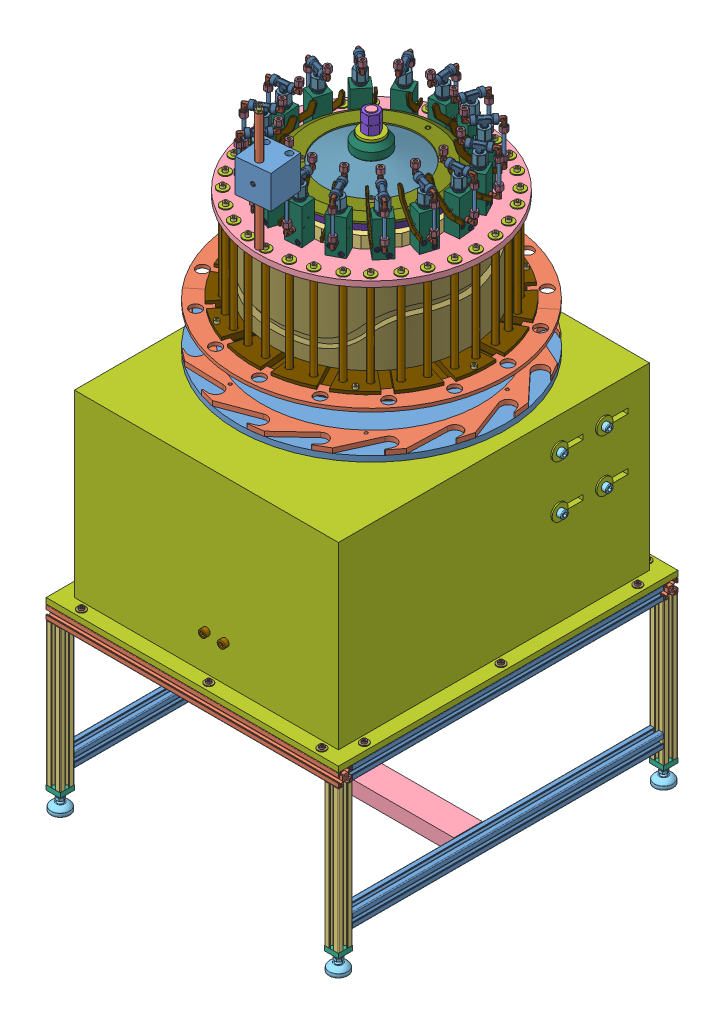
SolidWorks assembly Assieme_FINALE, configuration Default. Lengths in mm.
Overall size (1086.82 1425.57 1086.82).
701 component instances, 78 part files, 65 mates.
Components (placement in the parent):
- SupportoBase_Totale-2: SupportoBase_Totale [Default] at (4.0127 -14.4529 -3.9361) x (0 1 0) z (0 0 1) size (801.2 636.12 736.12)
  - Supporto_base_macchina-1: Supporto_base_macchina [Default] at origin size (378.2 636.12 736.12)
    - profilato_30x30_590-3: profilato_30x30_590 [Default] at (275.414 713.7262 -66.645) size (30 30 660)
    - profilato_30x30_590-5: profilato_30x30_590 [Default] at (275.414 123.7262 -66.645) size (30 30 660)
    - profilato_30x30_550-5: profilato_30x30_550 [Default] at (275.414 703.7262 -716.645) x (1 0 0) z (0 1 0) size (30 30 620)
    - profilato_30x30_550-6: profilato_30x30_550 [Default] at (275.414 703.7262 -26.645) x (1 0 0) z (0 1 0) size (30 30 620)
    - profilato_30x30_272-5: profilato_30x30_272 [Default] at (-16.586 123.7262 -716.645) x (0 0 1) z (-1 0 0) size (30 30 302)
    - profilato_30x30_272-6: profilato_30x30_272 [Default] at (-16.586 713.7262 -716.645) x (0 0 1) z (-1 0 0) size (30 30 302)
    - profilato_30x30_272-7: profilato_30x30_272 [Default] at (235.414 123.7262 -26.645) x (0 0 -1) z (1 0 0) size (30 30 302)
    - profilato_30x30_272-8: profilato_30x30_272 [Default] at (-16.586 713.7262 -26.645) x (0 0 1) z (-1 0 0) size (30 30 302)
    - profilo_U_60x30_490_supporto_base_macchina-1: profilo_U_60x30_490_supporto_base_macchina [Default] at (15.1 707.7262 -323.6583) x (0 0 1) z (0 -1 0) size (60 30 569)
    - profilato_30x30_590-6: profilato_30x30_590 [Default] at (3.414 123.7262 -66.645) size (30 30 660)
    - profilato_30x30_590-7: profilato_30x30_590 [Default] at (3.414 713.7262 -676.645) x (-1 0 0) z (0 0 -1) size (30 30 660)
    - 6322125-1: 6322125 [Default] at (-85.2818 713.7262 -26.645) x (0 0 -1) z (1 0 0) size (40 40 71.2)
    - 6322125-2: 6322125 [Default] at (-85.2818 713.7262 -716.645) x (0 0 -1) z (1 0 0) size (40 40 71.2)
    - 6322125-3: 6322125 [Default] at (-85.2818 123.7262 -26.645) x (0 -0.924225 -0.381849) z (1 0 0) size (40 40 71.2)
    - 6322125-4: 6322125 [Default] at (-85.2818 123.7262 -716.645) x (0 0 -1) z (1 0 0) size (40 40 71.2)
    - tappo_filettato_Supporto_base_macchina-1: tappo_filettato_Supporto_base_macchina [Default] at (-41.586 123.7262 -26.645) x (0 0 1) z (-1 0 0) size (30 30 10.37)
    - tappo_filettato_Supporto_base_macchina-2: tappo_filettato_Supporto_base_macchina [Default] at (-41.586 123.7262 -716.645) x (0 0 1) z (-1 0 0) size (30 30 10.37)
    - tappo_filettato_Supporto_base_macchina-3: tappo_filettato_Supporto_base_macchina [Default] at (-41.586 713.7262 -716.645) x (0 0 1) z (-1 0 0) size (30 30 10.37)
    - tappo_filettato_Supporto_base_macchina-4: tappo_filettato_Supporto_base_macchina [Default] at (-51.586 713.7262 -26.645) x (0 0 -1) z (1 0 0) size (30 30 10.37)
  - assieme_base-1: assieme_base [Default] at (466.8009 1138.7262 -472.0974) x (0 0 -1) z (0 -1 0) size (720 423 620)
    - Supporto di Base per macchina-1: Supporto di Base per macchina [Default] at (-460.4524 -176.3869 1030) size (720 403 620)
    - canotto di supporto-1: canotto di supporto [Default] at (-100.4524 134.8265 740) x (0 1 0) z (-0.866025 0 0.5) size (220 238 238)
    - m10 35mm-7: m10 35mm [ISO 4762 M10 x 35 - 35N] at (4.5476 246.6131 740) x (0 -1 0) z (1 0 0) size (45 16 16)
    - m10 35mm-8: m10 35mm [ISO 4762 M10 x 35 - 35N] at (-47.9524 246.6131 649.0673) x (0 -1 0) z (0.5 0 -0.866025) size (45 16 16)
    - m10 35mm-9: m10 35mm [ISO 4762 M10 x 35 - 35N] at (-152.9524 246.6131 649.0673) x (0 -1 0) z (-0.5 0 -0.866025) size (45 16 16)
    - m10 35mm-10: m10 35mm [ISO 4762 M10 x 35 - 35N] at (-205.4524 246.6131 740) x (0 -1 0) z (-1 0 0) size (45 16 16)
    - m10 35mm-11: m10 35mm [ISO 4762 M10 x 35 - 35N] at (-152.9524 246.6131 830.9327) x (0 -1 0) z (-0.5 0 0.866025) size (45 16 16)
    - m10 35mm-12: m10 35mm [ISO 4762 M10 x 35 - 35N] at (-47.9524 246.6131 830.9327) x (0 -1 0) z (0.5 0 0.866025) size (45 16 16)
    - Traversa di blocco albero-1: Traversa di blocco albero [Default] at (-100.4524 -86.3869 772.5) size (644 42 65)
    - m10 35mm-13: m10 35mm [ISO 4762 M10 x 35 - 35N] at (239.5476 -86.3869 760) x (-1 0 0) z (0 -1 0) size (45 16 16)
    - m10 35mm-16: m10 35mm [ISO 4762 M10 x 35 - 35N] at (239.5476 -86.3869 720) x (-1 0 0) z (0 -1 0) size (45 16 16)
    - m10 35mm-17: m10 35mm [ISO 4762 M10 x 35 - 35N] at (-440.4524 -86.3869 720) x (1 0 0) z (0 1 0) size (45 16 16)
    - m10 35mm-18: m10 35mm [ISO 4762 M10 x 35 - 35N] at (-440.4524 -86.3869 760) x (1 0 0) z (0 1 0) size (45 16 16)
  - DadoT-2: DadoT [Default] at (288.4104 668.7262 -716.645) x (0 0 -1) z (0 -1 0) size (16.5 6 8)
  - DadoT-9: DadoT [Default] at (288.4104 668.7262 -26.645) x (0 0 -1) z (0 -1 0) size (16.5 6 8)
  - DadoT-10: DadoT [Default] at (288.6104 713.7262 -661.645) x (0 1 0) z (0 0 -1) size (16.5 6 8)
  - DadoT-11: DadoT [Default] at (288.6104 713.7262 -371.645) x (0 1 0) z (0 0 -1) size (16.5 6 8)
  - DadoT-12: DadoT [Default] at (288.6104 713.7262 -81.645) x (0 1 0) z (0 0 -1) size (16.5 6 8)
  - DadoT-13: DadoT [Default] at (288.6104 123.7262 -661.645) x (0 1 0) z (0 0 -1) size (16.5 6 8)
  - DadoT-15: DadoT [Default] at (288.6104 123.7262 -371.645) x (0 1 0) z (0 0 -1) size (16.5 6 8)
  - DadoT-17: DadoT [Default] at (288.6104 123.7262 -81.645) x (0 1 0) z (0 0 -1) size (16.5 6 8)
  - RosettaM6-1: RosettaM6 [Washer ISO 7093 - 6] at (302.414 713.7262 -661.645) x (-1 0 0) z (0 0 1) size (1.6 18 18)
  - ViteM6-20-1: ViteM6-20 [ISO 4762 M6 x 20 - 20S] at (308.414 713.7262 -661.645) x (-1 0 0) z (0 0 1) size (26 10 10)
  - RosettaM6-2: RosettaM6 [Washer ISO 7093 - 6] at (302.414 668.7262 -716.645) x (-1 0 0) z (0 0 1) size (1.6 18 18)
  - ViteM6-20-2: ViteM6-20 [ISO 4762 M6 x 20 - 20S] at (308.414 668.7262 -716.645) x (-1 0 0) z (0 0 1) size (26 10 10)
  - RosettaM6-3: RosettaM6 [Washer ISO 7093 - 6] at (302.414 713.7262 -371.645) x (-1 0 0) z (0 0 1) size (1.6 18 18)
  - RosettaM6-4: RosettaM6 [Washer ISO 7093 - 6] at (302.414 713.7262 -81.645) x (-1 0 0) z (0 0 1) size (1.6 18 18)
  - ViteM6-20-3: ViteM6-20 [ISO 4762 M6 x 20 - 20S] at (308.414 713.7262 -371.645) x (-1 0 0) z (0 0 1) size (26 10 10)
  - ViteM6-20-4: ViteM6-20 [ISO 4762 M6 x 20 - 20S] at (308.414 713.7262 -81.645) x (-1 0 0) z (0 0 1) size (26 10 10)
  - RosettaM6-5: RosettaM6 [Washer ISO 7093 - 6] at (302.414 123.7262 -661.645) x (-1 0 0) z (0 0 1) size (1.6 18 18)
  - ViteM6-20-5: ViteM6-20 [ISO 4762 M6 x 20 - 20S] at (308.414 123.7262 -661.645) x (-1 0 0) z (0 0 1) size (26 10 10)
  - RosettaM6-6: RosettaM6 [Washer ISO 7093 - 6] at (302.414 123.7262 -371.645) x (-1 0 0) z (0 0 1) size (1.6 18 18)
  - RosettaM6-7: RosettaM6 [Washer ISO 7093 - 6] at (302.414 123.7262 -81.645) x (-1 0 0) z (0 0 1) size (1.6 18 18)
  - ViteM6-20-6: ViteM6-20 [ISO 4762 M6 x 20 - 20S] at (308.414 123.7262 -371.645) x (-1 0 0) z (0 0 1) size (26 10 10)
  - ViteM6-20-7: ViteM6-20 [ISO 4762 M6 x 20 - 20S] at (308.414 123.7262 -81.645) x (-1 0 0) z (0 0 1) size (26 10 10)
  - ViteM6-20-8: ViteM6-20 [ISO 4762 M6 x 20 - 20S] at (308.414 398.7262 -716.645) x (-1 0 0) z (0 0 1) size (26 10 10)
  - RosettaM6-8: RosettaM6 [Washer ISO 7093 - 6] at (302.414 398.7262 -716.645) x (-1 0 0) z (0 0 1) size (1.6 18 18)
  - DadoT-19: DadoT [Default] at (288.4104 398.7262 -716.645) x (0 0 -1) z (0 -1 0) size (16.5 6 8)
  - DadoT-20: DadoT [Default] at (288.4104 158.7262 -716.645) x (0 0 -1) z (0 -1 0) size (16.5 6 8)
  - RosettaM6-9: RosettaM6 [Washer ISO 7093 - 6] at (302.414 158.7262 -716.645) x (-1 0 0) z (0 0 1) size (1.6 18 18)
  - ViteM6-20-9: ViteM6-20 [ISO 4762 M6 x 20 - 20S] at (308.414 158.7262 -716.645) x (-1 0 0) z (0 0 1) size (26 10 10)
  - DadoT-21: DadoT [Default] at (288.4104 668.7262 -26.645) x (0 0 -1) z (0 -1 0) size (16.5 6 8)
  - RosettaM6-10: RosettaM6 [Washer ISO 7093 - 6] at (302.414 668.7262 -26.645) x (-1 0 0) z (0 0 1) size (1.6 18 18)
  - ViteM6-20-10: ViteM6-20 [ISO 4762 M6 x 20 - 20S] at (308.414 668.7262 -26.645) x (-1 0 0) z (0 0 1) size (26 10 10)
  - DadoT-22: DadoT [Default] at (288.4104 158.7262 -26.645) x (0 0 -1) z (0 -1 0) size (16.5 6 8)
  - RosettaM6-11: RosettaM6 [Washer ISO 7093 - 6] at (302.414 158.7262 -26.645) x (-1 0 0) z (0 0 1) size (1.6 18 18)
  - ViteM6-20-11: ViteM6-20 [ISO 4762 M6 x 20 - 20S] at (308.414 158.7262 -26.645) x (-1 0 0) z (0 0 1) size (26 10 10)
  - ViteM6-20-12: ViteM6-20 [ISO 4762 M6 x 20 - 20S] at (308.414 398.7262 -26.645) x (-1 0 0) z (0 0 1) size (26 10 10)
  - RosettaM6-12: RosettaM6 [Washer ISO 7093 - 6] at (302.414 398.7262 -26.645) x (-1 0 0) z (0 0 1) size (1.6 18 18)
  - DadoT-23: DadoT [Default] at (288.4104 398.7262 -26.645) x (0 0 -1) z (0 -1 0) size (16.5 6 8)
- motoriduttore-1: motoriduttore [Default] at (-164.7135 275.9611 -1137.0941) x (0 0 1) z (-1 0 0) size (200 160 175)
- Assieme_Riduttore-1: Assieme_Riduttore [Default] at (-58.5438 520.923 -522.9431) x (0 1 0) z (-0.993104 0 -0.117237) size (226 168.82 169.04)
  - AlberoRiduttore-1: AlberoRiduttore [Default] at (-61.6906 7.4655 211) size (201 29 29)
  - linguetta_uni6604_b_8x7x50-1: linguetta_uni6604_b_8x7x50 [Default] at (-116.7419 7.4655 226) x (1 0 0) z (0 1 0) size (50 7 8)
  - linguetta_uni6604_b_8x7x35-1: linguetta_uni6604_b_8x7x35 [Default] at (-33.7419 7.4655 226.5) x (1 0 0) z (0 1 0) size (35 7 8)
  - linguetta_uni6604_b_8x7x35-2: linguetta_uni6604_b_8x7x35 [Default] at (41.2581 7.4655 226.5) x (1 0 0) z (0 1 0) size (35 7 8)
  - ASSIEME-LASS-90-VERS-B-O-25-3D.step-1: ASSIEME-LASS-90-VERS-B-O-25-3D.step [Default] at (-111.3519 -70.5563 279.3493) x (-1 0 0) z (0 0.707107 -0.707107) size (64.28 105 105)
  - Rondella di fermo-1: Rondella di fermo [Default] at (-122.7419 7.4655 211) x (0 0.707107 -0.707107) z (-1 0 0) size (36 36 3)
  - M8 25 mm-1: M8 25 mm [ISO 4762 M8 x 25 - 25N] at (92.2581 7.4655 211) x (-1 0 0) z (0 1 0) size (33 13 13)
  - M8 25 mm-2: M8 25 mm [ISO 4762 M8 x 25 - 25N] at (-133.7419 7.4655 211) x (1 0 0) z (0 -0.707107 0.707107) size (33 13 13)
  - M6 16mm-3: M6 16mm [ISO 4762 M6 x 16 - 16N] at (-44.8119 40.5589 196.8286) x (-1 0 0) z (0 0.935687 0.352831) size (22 10 10)
  - M6 16mm-14: M6 16mm [ISO 4762 M6 x 16 - 16N] at (-44.8119 11.7394 175.2546) x (-1 0 0) z (0 0.773404 -0.633913) size (22 10 10)
  - M6 16mm-15: M6 16mm [ISO 4762 M6 x 16 - 16N] at (-44.8119 -21.354 189.426) x (-1 0 0) z (0 -0.162283 -0.986744) size (22 10 10)
  - M6 16mm-16: M6 16mm [ISO 4762 M6 x 16 - 16N] at (-44.8119 -25.6279 225.1714) x (-1 0 0) z (0 -0.935687 -0.352831) size (22 10 10)
  - M6 16mm-17: M6 16mm [ISO 4762 M6 x 16 - 16N] at (-44.8119 3.1916 246.7454) x (-1 0 0) z (0 -0.773404 0.633913) size (22 10 10)
  - M6 16mm-18: M6 16mm [ISO 4762 M6 x 16 - 16N] at (-44.8119 36.285 232.574) x (-1 0 0) z (0 0.162283 0.986744) size (22 10 10)
  - Parte1^Assieme_Riduttore-1: Parte1^Assieme_Riduttore [Default] at origin (virtual)
  - ruota dentata m22-4: ruota dentata m22 [Chain wheel ISO - 22Z 10A-1 --22SA36.0N] at (-59.7419 7.4655 211) x (1 0 0) z (0 -0.599278 0.800541) size (8.93 120.13 121.23)
  - Rondella di fermo-2: Rondella di fermo [Default] at (84.2581 7.4655 211) x (0 0 1) z (-1 0 0) size (36 36 3)
- M10 50mm-1: M10 50mm [ISO 4762 M10 x 50 - 50N] at (-121.7135 603.4611 -513.0941) x (-1 0 0) z (0 -0.924225 -0.381849) size (60 16 16)
- M10 50mm-2: M10 50mm [ISO 4762 M10 x 50 - 50N] at (-121.7135 492.4611 -513.0941) x (-1 0 0) z (0 0 1) size (60 16 16)
- M10 50mm-5: M10 50mm [ISO 4762 M10 x 50 - 50N] at (-121.7135 603.4611 -608.0941) x (-1 0 0) z (0 0 1) size (60 16 16)
- M10 50mm-4: M10 50mm [ISO 4762 M10 x 50 - 50N] at (-121.7135 492.4611 -608.0941) x (-1 0 0) z (0 0 1) size (60 16 16)
- DADO M10-9: DADO M10 [ISO - 4033 - M10 - W - N] at (-174.0135 603.4611 -608.0941) x (0 0 1) z (-1 0 0) size (16 18.48 9.3)
- DADO M10-8: DADO M10 [ISO - 4033 - M10 - W - N] at (-174.0135 603.4611 -513.0941) x (0 0 1) z (-1 0 0) size (16 18.48 9.3)
- DADO M10-7: DADO M10 [ISO - 4033 - M10 - W - N] at (-174.0135 492.4611 -608.0941) x (0 0 1) z (-1 0 0) size (16 18.48 9.3)
- DADO M10-10: DADO M10 [ISO - 4033 - M10 - W - N] at (-174.0135 492.4611 -513.0941) x (0 0 1) z (-1 0 0) size (16 18.48 9.3)
- rondella M10-9: rondella M10 [Washer ISO 7094 - 10] at (-134.7135 603.4611 -513.0941) x (-1 0 0) z (0 0.924225 0.381849) size (3 34 34)
- rondella M10-10: rondella M10 [Washer ISO 7094 - 10] at (-134.7135 492.4611 -513.0941) x (-1 0 0) z (0 0 1) size (3 34 34)
- rondella M10-12: rondella M10 [Washer ISO 7094 - 10] at (-134.7135 492.4611 -608.0941) x (-1 0 0) z (0 0 1) size (3 34 34)
- rondella M10-11: rondella M10 [Washer ISO 7094 - 10] at (-134.7135 603.4611 -608.0941) x (-1 0 0) z (0 0 1) size (3 34 34)
- catena_maschio-1: catena_maschio [Default] at (-321.9473 463.4961 -580.6395) x (-0.810007 0 0.58642) z (0 1 0) size (28.67 12.73 20.3)
- catena_femmina-1: catena_femmina [Default] at (-334.299 463.4961 -567.4631) x (0.810007 0 -0.58642) z (0 1 0) size (30.04 14.2 13.87)
  - ansi_50_02-1: ansi_50_02 [Default] at (17.7318 3.4296 0) x (1 0 0) z (0 0 -1) size (30.04 14.2 13.87)
  - ansi_50_03-1: ansi_50_03 [Default] at (17.7318 3.4296 -0.11) x (1 0 0) z (0 0 -1) size (10.16 10.16 9.46)
  - ansi_50_04-1: ansi_50_04 [Default] at (17.7318 3.4296 0.11) x (1 0 0) z (0 0 -1) size (10.16 10.16 9.46)
- rondella M8-1: rondella M8 [ISO 10673-9.3-S] at (-394.7135 376.9611 -360.5811) x (0 -1 0) z (-1 0 0) size (2 18 18)
- rondella M8-2: rondella M8 [ISO 10673-9.3-S] at (-394.7135 376.9611 -390.5811) x (0 -1 0) z (-1 0 0) size (2 18 18)
- M8 25 mm-1: M8 25 mm [ISO 4762 M8 x 25 - 25N] at (-394.7135 368.9611 -390.5811) x (0 1 0) z (0.5 0 0.866025) size (33 13 13)
- M8 25 mm-2: M8 25 mm [ISO 4762 M8 x 25 - 25N] at (-394.7135 366.9611 -360.5811) x (0 1 0) z (-0.5 0 -0.866025) size (33 13 13)
- assieme parte rotante-2: assieme parte rotante [Default] at (-79.201 623.9178 -645.7922) x (0 1 0) z (-0.73003 0 0.683415) size (749.63 778.63 778.63)
  - albero rotazione piatti-1: albero rotazione piatti [Default] at (60.413 18.3637 415) size (415 200 200)
  - seger 100mm-2: seger 100mm [KS 1336 E - 100] at (-146.4567 18.3637 415) x (0 0 -1) z (1 0 0) size (107.55 112.98 3)
  - SKF - 6020 - 20,DE,NC,20_68-1: SKF - 6020 - 20,DE,NC,20_68 [SKF - 6020 - 20,DE,NC,20_68] at (-131.4567 18.3637 415) x (1 0 0) z (0 -0.434476 -0.900684) size (24 150 150)
  - calettatore d95-1: calettatore d95 [Default] at (-173.8867 18.3637 415) size (39.5 135 135)
  - Chain wheel ISO - 50Z 10A-1-1: Chain wheel ISO - 50Z 10A-1 [Chain wheel ISO - 50Z 10A-1 --50SB120H25L95.0N] at (-164.8867 18.3637 415) size (28.93 262.06 262.51)
  - Disco supporto montaggio e Colonne-1: Disco supporto montaggio e Colonne [Default] at (204.0433 18.3637 415) x (0 -0.866025 -0.5) z (1 0 0) size (499.6 499.6 29)
  - SKF - 6020 - 20,DE,NC,20_68-2: SKF - 6020 - 20,DE,NC,20_68 [SKF - 6020 - 20,DE,NC,20_68] at (62.0433 18.3637 415) x (1 0 0) z (0 -0.432628 -0.901573) size (24 150 150)
  - piatto rotante porta tappi-1: piatto rotante porta tappi [Default] at (99.0433 18.3637 415) x (0 0 -1) z (1 0 0) size (570 570 20.57)
  - disco trasportatore tappi 31-1: disco trasportatore tappi 31 [Default] at (111.0433 18.3637 415) x (0 0.5 -0.866025) z (1 0 0) size (570 570 10.42)
  - Distributore Rotante-1: Distributore Rotante [Default] at (425.0433 18.3637 415) x (0 0.130526 -0.991445) z (1 0 0) size (310 310 25.54)
  - disco trascinato porta distributore vuoto-1: disco trascinato porta distributore vuoto [Default] at (400.0433 18.3637 415) x (0 -0.130526 0.991445) z (-1 0 0) size (480 480 50)
  - m12 35mm-1: m12 35mm [ISO 4762 M12 x 35 - 35N] at (376.0433 -45.1046 366.2991) x (1 0 0) z (0 -0.5 0.866025) size (47 18 18)
  - m12 90mm-3: m12 90mm [ISO 4762 M12 x 90 - 90N] at (203.0433 -21.6363 345.718) x (-1 0 0) z (0 -0.5 0.866025) size (102 18 18)
  - rondella M6-90: rondella M6 [Washer ISO 7094 - 6] at (99.0433 -101.6363 207.1539) x (1 0 0) z (0 -1 0) size (2 22 22)
  - M6 20mm-1: M6 20mm [ISO 4762 M6 x 20 - 20N] at (91.0433 -101.6363 207.1539) x (1 0 0) z (0 0.5 0.866025) size (26 10 10)
  - m12 35mm-2: m12 35mm [ISO 4762 M12 x 35 - 35N] at (376.0433 28.8058 335.6844) x (1 0 0) z (0 -1 0) size (47 18 18)
  - m12 35mm-3: m12 35mm [ISO 4762 M12 x 35 - 35N] at (376.0433 92.2741 384.3853) x (1 0 0) z (0 -0.5 -0.866025) size (47 18 18)
  - m12 35mm-4: m12 35mm [ISO 4762 M12 x 35 - 35N] at (376.0433 81.832 463.7009) x (1 0 0) z (0 0.5 -0.866025) size (47 18 18)
  - m12 35mm-5: m12 35mm [ISO 4762 M12 x 35 - 35N] at (376.0433 7.9216 494.3156) x (1 0 0) z (0 1 0) size (47 18 18)
  - m12 35mm-6: m12 35mm [ISO 4762 M12 x 35 - 35N] at (376.0433 -55.5467 445.6147) x (1 0 0) z (0 0.5 0.866025) size (47 18 18)
  - rondella M6-91: rondella M6 [Washer ISO 7094 - 6] at (99.0433 138.3637 207.1539) x (1 0 0) z (0 -0.5 -0.866025) size (2 22 22)
  - rondella M6-92: rondella M6 [Washer ISO 7094 - 6] at (99.0433 258.3637 415) x (1 0 0) z (0 0.5 -0.866025) size (2 22 22)
  - rondella M6-93: rondella M6 [Washer ISO 7094 - 6] at (99.0433 138.3637 622.8461) x (1 0 0) z (0 1 0) size (2 22 22)
  - rondella M6-94: rondella M6 [Washer ISO 7094 - 6] at (99.0433 -101.6363 622.8461) x (1 0 0) z (0 0.5 0.866025) size (2 22 22)
  - rondella M6-95: rondella M6 [Washer ISO 7094 - 6] at (99.0433 -221.6363 415) x (1 0 0) z (0 -0.5 0.866025) size (2 22 22)
  - M6 20mm-2: M6 20mm [ISO 4762 M6 x 20 - 20N] at (91.0433 138.3637 207.1539) x (1 0 0) z (0 -0.5 0.866025) size (26 10 10)
  - M6 20mm-3: M6 20mm [ISO 4762 M6 x 20 - 20N] at (91.0433 258.3637 415) x (1 0 0) z (0 -1 0) size (26 10 10)
  - M6 20mm-4: M6 20mm [ISO 4762 M6 x 20 - 20N] at (91.0433 138.3637 622.8461) x (1 0 0) z (0 -0.5 -0.866025) size (26 10 10)
  - M6 20mm-5: M6 20mm [ISO 4762 M6 x 20 - 20N] at (91.0433 -101.6363 622.8461) x (1 0 0) z (0 0.5 -0.866025) size (26 10 10)
  - M6 20mm-6: M6 20mm [ISO 4762 M6 x 20 - 20N] at (91.0433 -221.6363 415) x (1 0 0) z (0 1 0) size (26 10 10)
  - m12 90mm-4: m12 90mm [ISO 4762 M12 x 90 - 90N] at (203.0433 58.3637 345.718) x (-1 0 0) z (0 -1 0) size (102 18 18)
  - m12 90mm-5: m12 90mm [ISO 4762 M12 x 90 - 90N] at (203.0433 98.3637 415) x (-1 0 0) z (0 -0.5 -0.866025) size (102 18 18)
  - m12 90mm-6: m12 90mm [ISO 4762 M12 x 90 - 90N] at (203.0433 58.3637 484.282) x (-1 0 0) z (0 0.5 -0.866025) size (102 18 18)
  - m12 90mm-7: m12 90mm [ISO 4762 M12 x 90 - 90N] at (203.0433 -21.6363 484.282) x (-1 0 0) z (0 1 0) size (102 18 18)
  - m12 90mm-8: m12 90mm [ISO 4762 M12 x 90 - 90N] at (203.0433 -61.6363 415) x (-1 0 0) z (0 0.5 0.866025) size (102 18 18)
  - asta scorrimento carello-1: asta scorrimento carello [Default] at (287.5433 70.1437 197.9013) x (0 0 -1) z (1 0 0) size (12 12 225)
  - rondella M6-74: rondella M6 [Washer ISO 7094 - 6] at (175.0433 70.1437 197.9013) x (1 0 0) z (0 -1 0) size (2 22 22)
  - M6 16mm-1: M6 16mm [ISO 4762 M6 x 16 - 16N] at (167.0433 70.1437 197.9013) size (22 10 10)
  - M6 16mm-2: M6 16mm [ISO 4762 M6 x 16 - 16N] at (408.0433 70.1437 197.9013) x (-1 0 0) z (0 0 -1) size (22 10 10)
  - rondella M6-96: rondella M6 [Washer ISO 7094 - 6] at (400.0433 70.1437 197.9013) x (-1 0 0) z (0 1 0) size (2 22 22)
  - rondella M6-112: rondella M6 [Washer ISO 7094 - 6] at (175.0433 24.5373 191.8971) x (1 0 0) z (0 -0.965926 -0.258819) size (2 22 22)
  - M6 16mm-3: M6 16mm [ISO 4762 M6 x 16 - 16N] at (167.0433 24.5373 191.8971) x (1 0 0) z (0 0.258819 -0.965926) size (22 10 10)
  - asta scorrimento carello-2: asta scorrimento carello [Default] at (287.5433 24.5373 191.8971) x (0 0.258819 -0.965926) z (-1 0 0) size (12 12 225)
  - rondella M6-128: rondella M6 [Washer ISO 7094 - 6] at (400.0433 24.5373 191.8971) x (-1 0 0) z (0 0.965926 0.258819) size (2 22 22)
  - M6 16mm-4: M6 16mm [ISO 4762 M6 x 16 - 16N] at (408.0433 24.5373 191.8971) x (-1 0 0) z (0 -0.258819 0.965926) size (22 10 10)
  - AssiemeValvola-1: AssiemeValvola [Default] at (515.3257 103.3637 267.7757) x (0 -0.5 0.866025) z (0 0.866025 0.5) size (90.26 138.63 38)
    - RaccordoT-1: RaccordoT [Default] at origin size (43 29.75 16.5)
    - Raccordo a L-1: Raccordo a L [Default] at (-30 0 0) x (0 -1 0) z (0 0 -1) size (28.34 25.51 14.01)
      - 1809_06_10_01-1: 1809_06_10_01 [Default] at origin size (22.49 23 10)
      - 1809_06_10_02-1: 1809_06_10_02 [Default] at origin size (6.5 8.5 8.5)
      - 1809_06_10_03-1: 1809_06_10_03 [Default] at origin size (11.02 15.01 14.01)
    - Raccordo a L-2: Raccordo a L [Default] at (30 0 0) x (0 1 0) z (0 0 -1) size (28.34 25.51 14.01)
      - 1809_06_10_01-1: 1809_06_10_01 [Default] at origin size (22.49 23 10)
      - 1809_06_10_02-1: 1809_06_10_02 [Default] at origin size (6.5 8.5 8.5)
      - 1809_06_10_03-1: 1809_06_10_03 [Default] at origin size (11.02 15.01 14.01)
    - TappoChiusura-1: TappoChiusura [Default] at (0 -32 0) x (0 -1 0) z (0 0 1) size (38.28 26.74 26.74)
    - CorpoValvola-1: CorpoValvola [Default] at (-15 -115.2824 0) size (30 75 34)
    - Raccordo a L-3: Raccordo a L [Default] at (-30 -88.2824 0) x (0 1 0) z (0 0 1) size (28.34 25.51 14.01)
      - 1809_06_10_01-1: 1809_06_10_01 [Default] at origin size (22.49 23 10)
      - 1809_06_10_02-1: 1809_06_10_02 [Default] at origin size (6.5 8.5 8.5)
      - 1809_06_10_03-1: 1809_06_10_03 [Default] at origin size (11.02 15.01 14.01)
    - Spina_3x38-1: Spina_3x38 [Default] at (0 -68.2824 -21) x (-1 0 0) z (0 0 1) size (3 3 38)
    - Spina_3x38-2: Spina_3x38 [Default] at (-10 -80.2824 -21) x (0.996193 0.087174 0) z (0 0 1) size (3 3 38)
    - M5 40mm-3: M5 40mm [ISO 4762 M5 x 40 - 40N] at (-14.6 -108.7824 9) size (45 8.5 8.5)
    - M5 40mm-2: M5 40mm [ISO 4762 M5 x 40 - 40N] at (-14.6 -96.7824 -9) size (45 8.5 8.5)
    - LevaValvola-1: LevaValvola [Default] at (-24.507 -86.571 -17) x (0.996193 0.087174 0) z (0 0 1) size (77.55 60.2 4)
    - Tubo-1: Tubo [Default] at (-30 -15.9665 0) x (1 0 0) z (0 -1 0) size (6 6 56.4)
  - M6 16mm-5: M6 16mm [ISO 4762 M6 x 16 - 16N] at (167.0433 -16.8778 194.6116) x (1 0 0) z (0 0.382683 0.92388) size (22 10 10)
  - M6 16mm-6: M6 16mm [ISO 4762 M6 x 16 - 16N] at (167.0433 -98.5342 224.874) x (1 0 0) z (0 0.707107 0.707107) size (22 10 10)
  - M6 16mm-7: M6 16mm [ISO 4762 M6 x 16 - 16N] at (167.0433 -162.3939 284.0814) x (1 0 0) z (0 0.92388 0.382683) size (22 10 10)
  - M6 16mm-8: M6 16mm [ISO 4762 M6 x 16 - 16N] at (167.0433 -198.735 363.22) x (1 0 0) z (0 1 0) size (22 10 10)
  - M6 16mm-9: M6 16mm [ISO 4762 M6 x 16 - 16N] at (167.0433 -202.0247 450.2415) x (1 0 0) z (0 0.92388 -0.382683) size (22 10 10)
  - M6 16mm-10: M6 16mm [ISO 4762 M6 x 16 - 16N] at (167.0433 -171.7623 531.8979) x (1 0 0) z (0 0.707107 -0.707107) size (22 10 10)
  - M6 16mm-11: M6 16mm [ISO 4762 M6 x 16 - 16N] at (167.0433 -112.5549 595.7576) x (1 0 0) z (0 0.382683 -0.92388) size (22 10 10)
  - M6 16mm-12: M6 16mm [ISO 4762 M6 x 16 - 16N] at (167.0433 -33.4163 632.0987) x (1 0 0) z (0 0 -1) size (22 10 10)
  - M6 16mm-13: M6 16mm [ISO 4762 M6 x 16 - 16N] at (167.0433 53.6052 635.3884) x (1 0 0) z (0 -0.382683 -0.92388) size (22 10 10)
  - M6 16mm-14: M6 16mm [ISO 4762 M6 x 16 - 16N] at (167.0433 135.2616 605.126) x (1 0 0) z (0 -0.707107 -0.707107) size (22 10 10)
  - M6 16mm-15: M6 16mm [ISO 4762 M6 x 16 - 16N] at (167.0433 199.1213 545.9186) x (1 0 0) z (0 -0.92388 -0.382683) size (22 10 10)
  - M6 16mm-16: M6 16mm [ISO 4762 M6 x 16 - 16N] at (167.0433 235.4624 466.78) x (1 0 0) z (0 -1 0) size (22 10 10)
  - M6 16mm-17: M6 16mm [ISO 4762 M6 x 16 - 16N] at (167.0433 238.7521 379.7585) x (1 0 0) z (0 -0.92388 0.382683) size (22 10 10)
  - M6 16mm-18: M6 16mm [ISO 4762 M6 x 16 - 16N] at (167.0433 208.4897 298.1021) x (1 0 0) z (0 -0.707107 0.707107) size (22 10 10)
  - M6 16mm-19: M6 16mm [ISO 4762 M6 x 16 - 16N] at (167.0433 149.2823 234.2424) x (1 0 0) z (0 -0.382683 0.92388) size (22 10 10)
  - rondella M6-75: rondella M6 [Washer ISO 7094 - 6] at (175.0433 -16.8778 194.6116) x (1 0 0) z (0 -0.92388 0.382683) size (2 22 22)
  - rondella M6-76: rondella M6 [Washer ISO 7094 - 6] at (175.0433 -98.5342 224.874) x (1 0 0) z (0 -0.707107 0.707107) size (2 22 22)
  - rondella M6-77: rondella M6 [Washer ISO 7094 - 6] at (175.0433 -162.3939 284.0814) x (1 0 0) z (0 -0.382683 0.92388) size (2 22 22)
  - rondella M6-78: rondella M6 [Washer ISO 7094 - 6] at (175.0433 -198.735 363.22) size (2 22 22)
  - rondella M6-79: rondella M6 [Washer ISO 7094 - 6] at (175.0433 -202.0247 450.2415) x (1 0 0) z (0 0.382683 0.92388) size (2 22 22)
  - rondella M6-80: rondella M6 [Washer ISO 7094 - 6] at (175.0433 -171.7623 531.8979) x (1 0 0) z (0 0.707107 0.707107) size (2 22 22)
  - rondella M6-81: rondella M6 [Washer ISO 7094 - 6] at (175.0433 -112.5549 595.7576) x (1 0 0) z (0 0.92388 0.382683) size (2 22 22)
  - rondella M6-82: rondella M6 [Washer ISO 7094 - 6] at (175.0433 -33.4163 632.0987) x (1 0 0) z (0 1 0) size (2 22 22)
  - rondella M6-83: rondella M6 [Washer ISO 7094 - 6] at (175.0433 53.6052 635.3884) x (1 0 0) z (0 0.92388 -0.382683) size (2 22 22)
  - rondella M6-84: rondella M6 [Washer ISO 7094 - 6] at (175.0433 135.2616 605.126) x (1 0 0) z (0 0.707107 -0.707107) size (2 22 22)
  - rondella M6-85: rondella M6 [Washer ISO 7094 - 6] at (175.0433 199.1213 545.9186) x (1 0 0) z (0 0.382683 -0.92388) size (2 22 22)
  - rondella M6-86: rondella M6 [Washer ISO 7094 - 6] at (175.0433 235.4624 466.78) x (1 0 0) z (0 0 -1) size (2 22 22)
  - rondella M6-87: rondella M6 [Washer ISO 7094 - 6] at (175.0433 238.7521 379.7585) x (1 0 0) z (0 -0.382683 -0.92388) size (2 22 22)
  - rondella M6-88: rondella M6 [Washer ISO 7094 - 6] at (175.0433 208.4897 298.1021) x (1 0 0) z (0 -0.707107 -0.707107) size (2 22 22)
  - rondella M6-89: rondella M6 [Washer ISO 7094 - 6] at (175.0433 149.2823 234.2424) x (1 0 0) z (0 -0.92388 -0.382683) size (2 22 22)
  - asta scorrimento carello-3: asta scorrimento carello [Default] at (287.5433 -16.8778 194.6116) x (0 -0.382683 -0.92388) z (1 0 0) size (12 12 225)
  - asta scorrimento carello-4: asta scorrimento carello [Default] at (287.5433 -98.5342 224.874) x (0 -0.707107 -0.707107) z (1 0 0) size (12 12 225)
  - asta scorrimento carello-5: asta scorrimento carello [Default] at (287.5433 -162.3939 284.0814) x (0 -0.92388 -0.382683) z (1 0 0) size (12 12 225)
  - asta scorrimento carello-6: asta scorrimento carello [Default] at (287.5433 -198.735 363.22) x (0 -1 0) z (1 0 0) size (12 12 225)
  - asta scorrimento carello-7: asta scorrimento carello [Default] at (287.5433 -202.0247 450.2415) x (0 -0.92388 0.382683) z (1 0 0) size (12 12 225)
  - asta scorrimento carello-8: asta scorrimento carello [Default] at (287.5433 -171.7623 531.8979) x (0 -0.707107 0.707107) z (1 0 0) size (12 12 225)
  - asta scorrimento carello-9: asta scorrimento carello [Default] at (287.5433 -112.5549 595.7576) x (0 -0.382683 0.92388) z (1 0 0) size (12 12 225)
  - asta scorrimento carello-10: asta scorrimento carello [Default] at (287.5433 -33.4163 632.0987) x (0 0 1) z (1 0 0) size (12 12 225)
  - asta scorrimento carello-11: asta scorrimento carello [Default] at (287.5433 53.6052 635.3884) x (0 0.382683 0.92388) z (1 0 0) size (12 12 225)
  - asta scorrimento carello-12: asta scorrimento carello [Default] at (287.5433 135.2616 605.126) x (0 0.707107 0.707107) z (1 0 0) size (12 12 225)
  - asta scorrimento carello-13: asta scorrimento carello [Default] at (287.5433 199.1213 545.9186) x (0 0.92388 0.382683) z (1 0 0) size (12 12 225)
  - asta scorrimento carello-14: asta scorrimento carello [Default] at (287.5433 235.4624 466.78) x (0 1 0) z (1 0 0) size (12 12 225)
  - asta scorrimento carello-15: asta scorrimento carello [Default] at (287.5433 238.7521 379.7585) x (0 0.92388 -0.382683) z (1 0 0) size (12 12 225)
  - asta scorrimento carello-16: asta scorrimento carello [Default] at (287.5433 208.4897 298.1021) x (0 0.707107 -0.707107) z (1 0 0) size (12 12 225)
  - asta scorrimento carello-17: asta scorrimento carello [Default] at (287.5433 149.2823 234.2424) x (0 0.382683 -0.92388) z (1 0 0) size (12 12 225)
  - M6 16mm-20: M6 16mm [ISO 4762 M6 x 16 - 16N] at (408.0433 -16.8778 194.6116) x (-1 0 0) z (0 -0.382683 -0.92388) size (22 10 10)
  - M6 16mm-21: M6 16mm [ISO 4762 M6 x 16 - 16N] at (408.0433 -98.5342 224.874) x (-1 0 0) z (0 -0.707107 -0.707107) size (22 10 10)
  - M6 16mm-22: M6 16mm [ISO 4762 M6 x 16 - 16N] at (408.0433 -162.3939 284.0814) x (-1 0 0) z (0 -0.92388 -0.382683) size (22 10 10)
  - M6 16mm-23: M6 16mm [ISO 4762 M6 x 16 - 16N] at (408.0433 -198.735 363.22) x (-1 0 0) z (0 -1 0) size (22 10 10)
  - M6 16mm-24: M6 16mm [ISO 4762 M6 x 16 - 16N] at (408.0433 -202.0247 450.2415) x (-1 0 0) z (0 -0.92388 0.382683) size (22 10 10)
  - M6 16mm-25: M6 16mm [ISO 4762 M6 x 16 - 16N] at (408.0433 -171.7623 531.8979) x (-1 0 0) z (0 -0.707107 0.707107) size (22 10 10)
  - M6 16mm-26: M6 16mm [ISO 4762 M6 x 16 - 16N] at (408.0433 -112.5549 595.7576) x (-1 0 0) z (0 -0.382683 0.92388) size (22 10 10)
  - M6 16mm-27: M6 16mm [ISO 4762 M6 x 16 - 16N] at (408.0433 -33.4163 632.0987) x (-1 0 0) z (0 0 1) size (22 10 10)
  - M6 16mm-28: M6 16mm [ISO 4762 M6 x 16 - 16N] at (408.0433 53.6052 635.3884) x (-1 0 0) z (0 0.382683 0.92388) size (22 10 10)
  - M6 16mm-29: M6 16mm [ISO 4762 M6 x 16 - 16N] at (408.0433 135.2616 605.126) x (-1 0 0) z (0 0.707107 0.707107) size (22 10 10)
  - M6 16mm-30: M6 16mm [ISO 4762 M6 x 16 - 16N] at (408.0433 199.1213 545.9186) x (-1 0 0) z (0 0.92388 0.382683) size (22 10 10)
  - M6 16mm-31: M6 16mm [ISO 4762 M6 x 16 - 16N] at (408.0433 235.4624 466.78) x (-1 0 0) z (0 1 0) size (22 10 10)
  - M6 16mm-32: M6 16mm [ISO 4762 M6 x 16 - 16N] at (408.0433 238.7521 379.7585) x (-1 0 0) z (0 0.92388 -0.382683) size (22 10 10)
  - M6 16mm-33: M6 16mm [ISO 4762 M6 x 16 - 16N] at (408.0433 208.4897 298.1021) x (-1 0 0) z (0 0.707107 -0.707107) size (22 10 10)
  - M6 16mm-34: M6 16mm [ISO 4762 M6 x 16 - 16N] at (408.0433 149.2823 234.2424) x (-1 0 0) z (0 0.382683 -0.92388) size (22 10 10)
  - rondella M6-97: rondella M6 [Washer ISO 7094 - 6] at (400.0433 -16.8778 194.6116) x (-1 0 0) z (0 0.92388 -0.382683) size (2 22 22)
  - rondella M6-98: rondella M6 [Washer ISO 7094 - 6] at (400.0433 -98.5342 224.874) x (-1 0 0) z (0 0.707107 -0.707107) size (2 22 22)
  - rondella M6-99: rondella M6 [Washer ISO 7094 - 6] at (400.0433 -162.3939 284.0814) x (-1 0 0) z (0 0.382683 -0.92388) size (2 22 22)
  - rondella M6-100: rondella M6 [Washer ISO 7094 - 6] at (400.0433 -198.735 363.22) x (-1 0 0) z (0 0 -1) size (2 22 22)
  - rondella M6-101: rondella M6 [Washer ISO 7094 - 6] at (400.0433 -202.0247 450.2415) x (-1 0 0) z (0 -0.382683 -0.92388) size (2 22 22)
  - rondella M6-102: rondella M6 [Washer ISO 7094 - 6] at (400.0433 -171.7623 531.8979) x (-1 0 0) z (0 -0.707107 -0.707107) size (2 22 22)
  - rondella M6-103: rondella M6 [Washer ISO 7094 - 6] at (400.0433 -112.5549 595.7576) x (-1 0 0) z (0 -0.92388 -0.382683) size (2 22 22)
  - rondella M6-104: rondella M6 [Washer ISO 7094 - 6] at (400.0433 -33.4163 632.0987) x (-1 0 0) z (0 -1 0) size (2 22 22)
  - rondella M6-105: rondella M6 [Washer ISO 7094 - 6] at (400.0433 53.6052 635.3884) x (-1 0 0) z (0 -0.92388 0.382683) size (2 22 22)
  - rondella M6-106: rondella M6 [Washer ISO 7094 - 6] at (400.0433 135.2616 605.126) x (-1 0 0) z (0 -0.707107 0.707107) size (2 22 22)
  - rondella M6-107: rondella M6 [Washer ISO 7094 - 6] at (400.0433 199.1213 545.9186) x (-1 0 0) z (0 -0.382683 0.92388) size (2 22 22)
  - rondella M6-108: rondella M6 [Washer ISO 7094 - 6] at (400.0433 235.4624 466.78) x (-1 0 0) z (0 0 1) size (2 22 22)
  - rondella M6-109: rondella M6 [Washer ISO 7094 - 6] at (400.0433 238.7521 379.7585) x (-1 0 0) z (0 0.382683 0.92388) size (2 22 22)
  - rondella M6-110: rondella M6 [Washer ISO 7094 - 6] at (400.0433 208.4897 298.1021) x (-1 0 0) z (0 0.707107 0.707107) size (2 22 22)
  - rondella M6-111: rondella M6 [Washer ISO 7094 - 6] at (400.0433 149.2823 234.2424) x (-1 0 0) z (0 0.92388 0.382683) size (2 22 22)
  - rondella M6-113: rondella M6 [Washer ISO 7094 - 6] at (175.0433 -61.3104 206.5173) x (1 0 0) z (0 -0.991445 0.130526) size (2 22 22)
  - rondella M6-114: rondella M6 [Washer ISO 7094 - 6] at (175.0433 -135.0285 252.8771) x (1 0 0) z (0 -0.866025 0.5) size (2 22 22)
  - rondella M6-115: rondella M6 [Washer ISO 7094 - 6] at (175.0433 -185.3939 323.9186) x (1 0 0) z (0 -0.608761 0.793353) size (2 22 22)
  - rondella M6-116: rondella M6 [Washer ISO 7094 - 6] at (175.0433 -204.7392 408.8264) x (1 0 0) z (0 -0.258819 0.965926) size (2 22 22)
  - rondella M6-117: rondella M6 [Washer ISO 7094 - 6] at (175.0433 -190.119 494.6741) x (1 0 0) z (0 0.130526 0.991445) size (2 22 22)
  - rondella M6-118: rondella M6 [Washer ISO 7094 - 6] at (175.0433 -143.7592 568.3922) x (1 0 0) z (0 0.5 0.866025) size (2 22 22)
  - rondella M6-119: rondella M6 [Washer ISO 7094 - 6] at (175.0433 -72.7177 618.7576) x (1 0 0) z (0 0.793353 0.608761) size (2 22 22)
  - rondella M6-120: rondella M6 [Washer ISO 7094 - 6] at (175.0433 12.1901 638.1029) x (1 0 0) z (0 0.965926 0.258819) size (2 22 22)
  - rondella M6-121: rondella M6 [Washer ISO 7094 - 6] at (175.0433 98.0378 623.4827) x (1 0 0) z (0 0.991445 -0.130526) size (2 22 22)
  - rondella M6-122: rondella M6 [Washer ISO 7094 - 6] at (175.0433 171.7559 577.1229) x (1 0 0) z (0 0.866025 -0.5) size (2 22 22)
  - rondella M6-123: rondella M6 [Washer ISO 7094 - 6] at (175.0433 222.1213 506.0814) x (1 0 0) z (0 0.608761 -0.793353) size (2 22 22)
  - rondella M6-124: rondella M6 [Washer ISO 7094 - 6] at (175.0433 241.4666 421.1736) x (1 0 0) z (0 0.258819 -0.965926) size (2 22 22)
  - rondella M6-125: rondella M6 [Washer ISO 7094 - 6] at (175.0433 226.8464 335.3259) x (1 0 0) z (0 -0.130526 -0.991445) size (2 22 22)
  - rondella M6-126: rondella M6 [Washer ISO 7094 - 6] at (175.0433 180.4866 261.6078) x (1 0 0) z (0 -0.5 -0.866025) size (2 22 22)
  - rondella M6-127: rondella M6 [Washer ISO 7094 - 6] at (175.0433 109.4451 211.2424) x (1 0 0) z (0 -0.793353 -0.608761) size (2 22 22)
  - M6 16mm-35: M6 16mm [ISO 4762 M6 x 16 - 16N] at (167.0433 -61.3104 206.5173) x (1 0 0) z (0 -0.130526 -0.991445) size (22 10 10)
  - M6 16mm-36: M6 16mm [ISO 4762 M6 x 16 - 16N] at (167.0433 -135.0285 252.8771) x (1 0 0) z (0 -0.5 -0.866025) size (22 10 10)
  - M6 16mm-37: M6 16mm [ISO 4762 M6 x 16 - 16N] at (167.0433 -185.3939 323.9186) x (1 0 0) z (0 -0.793353 -0.608761) size (22 10 10)
  - M6 16mm-38: M6 16mm [ISO 4762 M6 x 16 - 16N] at (167.0433 -204.7392 408.8264) x (1 0 0) z (0 -0.965926 -0.258819) size (22 10 10)
  - M6 16mm-39: M6 16mm [ISO 4762 M6 x 16 - 16N] at (167.0433 -190.119 494.6741) x (1 0 0) z (0 -0.991445 0.130526) size (22 10 10)
  - M6 16mm-40: M6 16mm [ISO 4762 M6 x 16 - 16N] at (167.0433 -143.7592 568.3922) x (1 0 0) z (0 -0.866025 0.5) size (22 10 10)
  - M6 16mm-41: M6 16mm [ISO 4762 M6 x 16 - 16N] at (167.0433 -72.7177 618.7576) x (1 0 0) z (0 -0.608761 0.793353) size (22 10 10)
  - M6 16mm-42: M6 16mm [ISO 4762 M6 x 16 - 16N] at (167.0433 12.1901 638.1029) x (1 0 0) z (0 -0.258819 0.965926) size (22 10 10)
  - M6 16mm-43: M6 16mm [ISO 4762 M6 x 16 - 16N] at (167.0433 98.0378 623.4827) x (1 0 0) z (0 0.130526 0.991445) size (22 10 10)
  - M6 16mm-44: M6 16mm [ISO 4762 M6 x 16 - 16N] at (167.0433 171.7559 577.1229) x (1 0 0) z (0 0.5 0.866025) size (22 10 10)
  - M6 16mm-45: M6 16mm [ISO 4762 M6 x 16 - 16N] at (167.0433 222.1213 506.0814) x (1 0 0) z (0 0.793353 0.608761) size (22 10 10)
  - M6 16mm-46: M6 16mm [ISO 4762 M6 x 16 - 16N] at (167.0433 241.4666 421.1736) x (1 0 0) z (0 0.965926 0.258819) size (22 10 10)
  - M6 16mm-47: M6 16mm [ISO 4762 M6 x 16 - 16N] at (167.0433 226.8464 335.3259) x (1 0 0) z (0 0.991445 -0.130526) size (22 10 10)
  - M6 16mm-48: M6 16mm [ISO 4762 M6 x 16 - 16N] at (167.0433 180.4866 261.6078) x (1 0 0) z (0 0.866025 -0.5) size (22 10 10)
  - M6 16mm-49: M6 16mm [ISO 4762 M6 x 16 - 16N] at (167.0433 109.4451 211.2424) x (1 0 0) z (0 0.608761 -0.793353) size (22 10 10)
